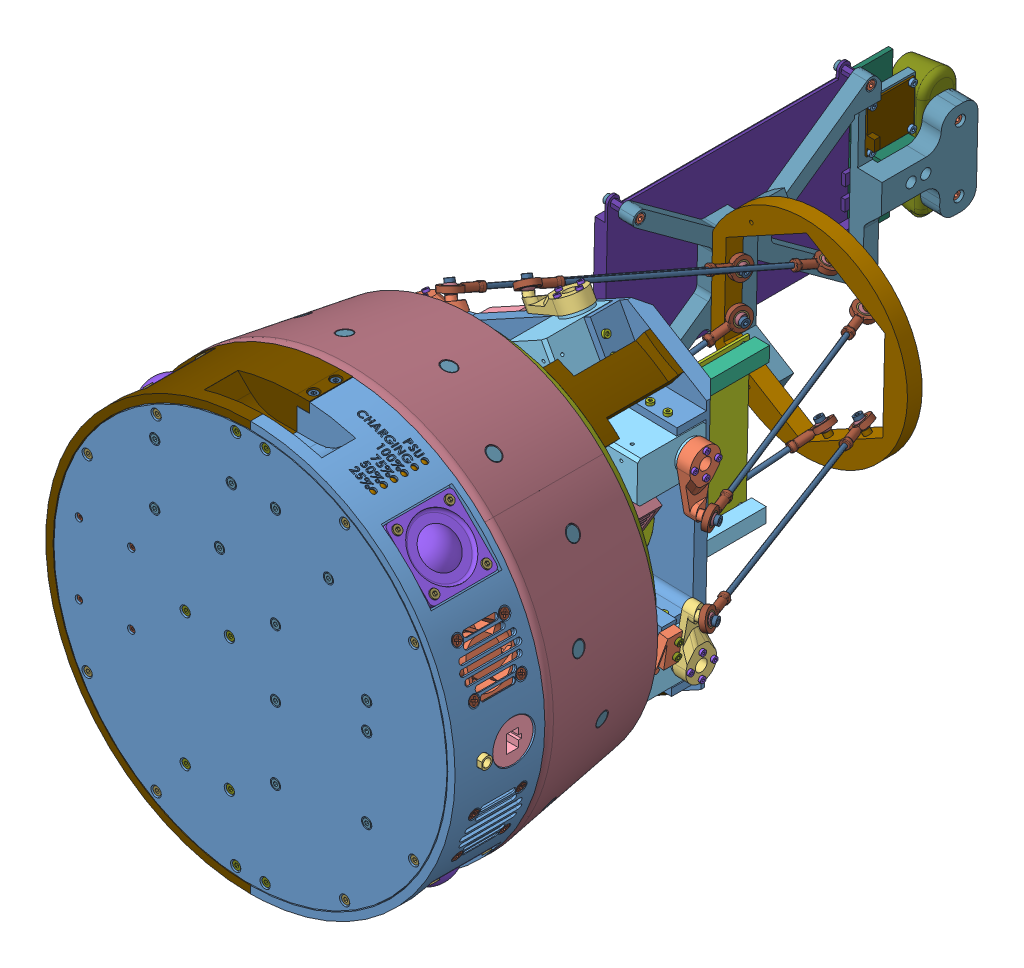
SolidWorks assembly robot, configuration Défaut. Lengths in mm.
Overall size (396.47 396.47 545.77).
549 component instances, 74 part files, 32 mates.
Components (placement in the parent):
- base-1: base [Défaut] at (1.1221 6.1042 181.6948) size (396.47 396.47 151)
  - base disk-1: base disk [Défaut] at (-2.864 19.6864 20.1) size (267 267 64.2)
    - base disk-1: base disk [Défaut] at (-39.9498 -9.3034 266.18) size (267 267 4)
    - Adafruit MAX9744-1: Adafruit MAX9744 [Défaut] at (-138.6977 -9.3034 256.18) x (0 1 0) z (0 0 -1) size (56.74 43.64 13.6)
    - Adafruit MAX9744-2: Adafruit MAX9744 [Défaut] at (-138.6977 -9.3034 239.58) x (0 1 0) z (0 0 -1) size (56.74 43.64 13.6)
    - Battery charger RRC-PMM240-1: Battery charger RRC-PMM240 [Défaut] at (-49.1471 67.1868 256.18) x (0 -1 0) z (0 0 -1) size (57 70 12)
    - battery holder-1: battery holder [Défaut] at (-89.2498 0.6966 266.18) x (0 -1 0) z (1 0 0) size (100 10 40)
    - Battery RRC2054-2-1: Battery RRC2054-2 [Défaut] at (-78.6791 -10.7125 233.18) x (0 1 0) z (0 0 1) size (151 78 23)
    - ground loop noise isolator-1: ground loop noise isolator [Défaut] at (-101.4098 -100.3034 233.18) x (0 -1 0) z (1 0 0) size (20 20 60)
    - ground loop noise isolator-2: ground loop noise isolator [Défaut] at (-41.4098 -80.3034 233.18) x (0 0 1) z (-1 0 0) size (20 20 60)
    - psu control-1: psu control [Défaut] at (-26.9498 90.6966 256.18) x (0 -1 0) z (0 0 -1) size (90 70 19.1)
    - buck boost-2: buck boost [Défaut] at (-26.9498 -9.3034 229.58) x (0 -1 0) z (0 0 -1) size (80 70 23.6)
    - 732-12936-ND-1: 732-12936-ND [Défaut] at (-156.4777 14.8266 254.58) x (-0.923728 -0.383049 0) z (0 0 -1) size (4.6 4.17 20)
    - 732-12936-ND-2: 732-12936-ND [Défaut] at (-156.4777 -33.4334 254.58) x (-0.923728 -0.383049 0) z (0 0 -1) size (4.6 4.17 20)
    - 732-12936-ND-3: 732-12936-ND [Défaut] at (-120.9177 -33.4334 254.58) x (-0.923728 -0.383049 0) z (0 0 -1) size (4.6 4.17 20)
    - 732-12936-ND-4: 732-12936-ND [Défaut] at (-120.9177 14.8266 254.58) x (-0.923728 -0.383049 0) z (0 0 -1) size (4.6 4.17 20)
    - 732-12918-ND-1: 732-12918-ND [Défaut] at (-156.4777 14.8266 266.18) x (-0.923728 -0.383049 0) z (0 0 -1) size (4.6 4.17 15)
    - 732-12918-ND-2: 732-12918-ND [Défaut] at (-120.9177 14.8266 266.18) x (-0.923728 -0.383049 0) z (0 0 -1) size (4.6 4.17 15)
    - 732-12918-ND-3: 732-12918-ND [Défaut] at (-120.9177 -33.4334 266.18) x (-0.923728 -0.383049 0) z (0 0 -1) size (4.6 4.17 15)
    - 732-12918-ND-4: 732-12918-ND [Défaut] at (-156.4777 -33.4334 266.18) x (-0.923728 -0.383049 0) z (0 0 -1) size (4.6 4.17 15)
    - M2x5mm socket-1: M2x5mm socket [Défaut] at (-156.4777 -33.4334 262.68) size (3.8 3.8 6.6)
    - M2x5mm socket-2: M2x5mm socket [Défaut] at (-120.9177 -33.4334 262.68) size (3.8 3.8 6.6)
    - M2x5mm socket-3: M2x5mm socket [Défaut] at (-156.4777 14.8266 262.68) size (3.8 3.8 6.6)
    - M2x5mm socket-4: M2x5mm socket [Défaut] at (-120.9177 14.8266 262.68) size (3.8 3.8 6.6)
    - M2 nut-1: M2 nut [Défaut] at (-156.4777 14.8266 237.98) x (-0.923728 -0.383049 0) z (0 0 -1) size (4.62 4 1.6)
    - M2 nut-2: M2 nut [Défaut] at (-156.4777 -33.4334 237.98) x (-0.923728 -0.383049 0) z (0 0 -1) size (4.62 4 1.6)
    - M2 nut-3: M2 nut [Défaut] at (-120.9177 -33.4334 237.98) x (-0.923728 -0.383049 0) z (0 0 -1) size (4.62 4 1.6)
    - M2 nut-4: M2 nut [Défaut] at (-120.9177 14.8266 237.98) x (-0.923728 -0.383049 0) z (0 0 -1) size (4.62 4 1.6)
    - 36-24337-ND-1: 36-24337-ND [Défaut] at (-104.9498 86.6966 266.18) x (-0.923728 -0.383049 0) z (0 0 -1) size (5.77 5 18)
    - 36-24337-ND-2: 36-24337-ND [Défaut] at (-104.9498 45.6966 266.18) x (-0.923728 -0.383049 0) z (0 0 -1) size (5.77 5 18)
    - 36-24337-ND-3: 36-24337-ND [Défaut] at (-60.9498 44.6966 266.18) x (-0.923728 -0.383049 0) z (0 0 -1) size (5.77 5 18)
    - 36-24337-ND-4: 36-24337-ND [Défaut] at (-52.9498 86.6966 266.18) x (-0.923728 -0.383049 0) z (0 0 -1) size (5.77 5 18)
    - M3x5mm socket-1: M3x5mm socket [Défaut] at (-104.9498 86.6966 262.18) size (5.5 5.5 8)
    - M3x5mm socket-2: M3x5mm socket [Défaut] at (-104.9498 45.6966 262.18) size (5.5 5.5 8)
    - M3x5mm socket-3: M3x5mm socket [Défaut] at (-60.9498 44.6966 262.18) size (5.5 5.5 8)
    - M3x5mm socket-4: M3x5mm socket [Défaut] at (-52.9498 86.6966 262.18) size (5.5 5.5 8)
    - M3 nut-1: M3 nut [Défaut] at (-104.9498 86.6966 254.18) x (-0.923728 -0.383049 0) z (0 0 -1) size (6.35 5.5 2.4)
    - M3 nut-2: M3 nut [Défaut] at (-104.9498 45.6966 254.18) x (-0.923728 -0.383049 0) z (0 0 -1) size (6.35 5.5 2.4)
    - M3 nut-3: M3 nut [Défaut] at (-60.9498 44.6966 254.18) x (-0.923728 -0.383049 0) z (0 0 -1) size (6.35 5.5 2.4)
    - M3 nut-4: M3 nut [Défaut] at (-52.9498 86.6966 254.18) x (-0.923728 -0.383049 0) z (0 0 -1) size (6.35 5.5 2.4)
    - M3x5mm plastic-1: M3x5mm plastic [Défaut] at (-84.2498 -94.3034 262.18) size (5.5 5.5 7.3)
    - M3x5mm plastic-2: M3x5mm plastic [Défaut] at (-84.2498 -4.3034 262.18) size (5.5 5.5 7.3)
    - M3x5mm plastic-3: M3x5mm plastic [Défaut] at (-54.2498 -94.3034 262.18) size (5.5 5.5 7.3)
    - M3x5mm plastic-4: M3x5mm plastic [Défaut] at (-54.2498 -4.3034 262.18) size (5.5 5.5 7.3)
    - 36-24337-ND-5: 36-24337-ND [Défaut] at (-22.9498 86.6966 266.18) x (-0.923728 -0.383049 0) z (0 0 -1) size (5.77 5 18)
    - 36-24337-ND-6: 36-24337-ND [Défaut] at (-22.9498 18.6966 266.18) x (-1 0 0) z (0 0 -1) size (5.77 5 18)
    - 36-24337-ND-7: 36-24337-ND [Défaut] at (13.0502 63.6966 266.18) x (-0.923728 -0.383049 0) z (0 0 -1) size (5.77 5 18)
    - 36-24337-ND-8: 36-24337-ND [Défaut] at (39.0502 4.6966 266.18) x (-1 0 0) z (0 0 -1) size (5.77 5 18)
    - M3x5mm socket-5: M3x5mm socket [Défaut] at (-22.9498 86.6966 262.18) size (5.5 5.5 8)
    - M3x5mm socket-6: M3x5mm socket [Défaut] at (13.0502 63.6966 262.18) size (5.5 5.5 8)
    - M3x5mm socket-7: M3x5mm socket [Défaut] at (39.0502 4.6966 262.18) size (5.5 5.5 8)
    - M3x5mm socket-8: M3x5mm socket [Défaut] at (-22.9498 18.6966 262.18) size (5.5 5.5 8)
    - M3 nut-5: M3 nut [Défaut] at (-22.9498 86.6966 252.18) size (6.35 5.5 2.4)
    - M3 nut-6: M3 nut [Défaut] at (13.0502 63.6966 252.18) size (6.35 5.5 2.4)
    - M3 nut-7: M3 nut [Défaut] at (-22.9498 18.6966 252.18) size (6.35 5.5 2.4)
    - M3 nut-8: M3 nut [Défaut] at (39.0502 4.6966 252.18) size (6.35 5.5 2.4)
    - 36-24337-ND-9: 36-24337-ND [Défaut] at (-22.9498 -26.3034 266.18) x (-0.923728 -0.383049 0) z (0 0 -1) size (5.77 5 18)
    - 36-24337-ND-10: 36-24337-ND [Défaut] at (-22.9498 -75.3034 266.18) x (-0.923728 -0.383049 0) z (0 0 -1) size (5.77 5 18)
    - 36-24337-ND-11: 36-24337-ND [Défaut] at (39.0502 -67.3034 266.18) x (-0.923728 -0.383049 0) z (0 0 -1) size (5.77 5 18)
    - 36-24337-ND-12: 36-24337-ND [Défaut] at (39.0502 -13.3034 266.18) x (-0.923728 -0.383049 0) z (0 0 -1) size (5.77 5 18)
    - M3x5mm socket-9: M3x5mm socket [Défaut] at (39.0502 -13.3034 262.18) x (0.878614 0.477533 0) z (0 0 1) size (5.5 5.5 8)
    - M3x5mm socket-10: M3x5mm socket [Défaut] at (39.0502 -67.3034 262.18) size (5.5 5.5 8)
    - M3x5mm socket-11: M3x5mm socket [Défaut] at (-22.9498 -75.3034 262.18) size (5.5 5.5 8)
    - M3x5mm socket-12: M3x5mm socket [Défaut] at (-22.9498 -26.3034 262.18) size (5.5 5.5 8)
    - buck boost-1: buck boost [Défaut] at (-26.9498 -9.3034 256.18) x (0 -1 0) z (0 0 -1) size (80 70 23.6)
    - 36-24342-ND-1: 36-24342-ND [Défaut] at (-22.9498 -26.3034 254.58) x (1 0 0) z (0 0 -1) size (5.77 5 33)
    - 36-24342-ND-2: 36-24342-ND [Défaut] at (-22.9498 -75.3034 254.58) x (1 0 0) z (0 0 -1) size (5.77 5 33)
    - 36-24342-ND-3: 36-24342-ND [Défaut] at (39.0502 -13.3034 254.58) x (1 0 0) z (0 0 -1) size (5.77 5 33)
    - 36-24342-ND-4: 36-24342-ND [Défaut] at (39.0502 -67.3034 254.58) x (1 0 0) z (0 0 -1) size (5.77 5 33)
    - M3 nut-9: M3 nut [Défaut] at (39.0502 -13.3034 225.58) size (6.35 5.5 2.4)
    - M3 nut-10: M3 nut [Défaut] at (-22.9498 -26.3034 225.58) size (6.35 5.5 2.4)
    - M3 nut-11: M3 nut [Défaut] at (-22.9498 -75.3034 225.58) size (6.35 5.5 2.4)
    - M3 nut-12: M3 nut [Défaut] at (39.0502 -67.3034 225.58) size (6.35 5.5 2.4)
  - base audio-1: base audio [Défaut] at (-124.8488 -53.3863 500.7234) x (-0.707186 -0.707027 0) z (0 0 -1) size (280.35 280.35 66)
    - base audio 1-1: base audio 1 [Défaut] at (-103.1006 -12.9042 210.4434) size (243.44 238.72 66)
    - base audio 2-1: base audio 2 [Défaut] at (-103.1006 -12.9042 210.4434) size (237.43 237.43 66)
    - Noctua NF-A4X20-1: Noctua NF-A4X20 [Défaut] at (-150.4017 -116.7762 243.4434) x (0.910081 -0.414431 0) z (-0.414431 -0.910081 0) size (39.9 39.9 19.95)
    - Noctua NF-A4X20-2: Noctua NF-A4X20 [Défaut] at (-206.9702 -60.2108 243.4434) x (0 0 1) z (-0.910059 -0.414479 0) size (39.9 39.9 19.95)
    - SC2073-ND-1: SC2073-ND [Défaut] at (-196.9231 -106.7266 228.7434) x (-0.707107 0.707107 0) z (-0.707107 -0.707107 0) size (11.94 11.94 36.36)
    - RJ45 connector-1: RJ45 connector [Défaut] at (-200.7415 -110.545 250.4434) x (-0.707107 0.707107 0) z (0.707107 0.707107 0) size (27.9 27.9 35.9)
    - switch-1: switch [Défaut] at (-57.531 -144.4179 258.9434) x (0.944885 0.327404 0) z (-0.327404 0.944885 0) size (20.75 14.7 24.67)
    - Micro USB B (Adafruit 4217)-1: Micro USB B (Adafruit 4217) [Défaut] at (-68.5317 -112.6698 234.4434) x (0.944885 0.327404 0) z (0 0 -1) size (28 33.5 28)
    - Micro USB B nut (Adafruit 4217)-1: Micro USB B nut (Adafruit 4217) [Défaut] at (-60.3466 -136.2919 234.4434) x (0.892807 0.309359 0.327404) z (-0.327404 0.944885 0) size (30.02 30.02 8)
    - Dayton Audio DMA45-8-1: Dayton Audio DMA45-8 [Défaut] at (-103.1023 -147.0792 243.4417) x (1 0 0) z (0 -1 0) size (46 46 32.1)
    - LED 5mm-1: LED 5mm [Défaut] at (-235.7284 26.7015 262.9434) x (-0.32152 -0.927903 0.188734) z (0.944885 -0.327404 0) size (5.5 5.5 18.7)
    - LED 5mm-2: LED 5mm [Défaut] at (-235.7284 26.7015 227.9434) x (-0.107193 -0.309359 0.944885) z (0.944885 -0.327404 0) size (5.5 5.5 18.7)
    - LED 5mm-3: LED 5mm [Défaut] at (-235.7284 26.7015 255.9434) x (-0.107193 -0.309359 0.944885) z (0.944885 -0.327404 0) size (5.5 5.5 18.7)
    - LED 5mm-4: LED 5mm [Défaut] at (-235.7284 26.7015 248.9434) x (-0.107193 -0.309359 0.944885) z (0.944885 -0.327404 0) size (5.5 5.5 18.7)
    - LED 5mm-5: LED 5mm [Défaut] at (-235.7284 26.7015 241.9434) x (-0.107193 -0.309359 0.944885) z (0.944885 -0.327404 0) size (5.5 5.5 18.7)
    - LED 5mm-6: LED 5mm [Défaut] at (-235.7284 26.7015 234.9434) x (-0.107193 -0.309359 0.944885) z (0.944885 -0.327404 0) size (5.5 5.5 18.7)
    - M3x12mm plastic-1: M3x12mm plastic [Défaut] at (-193.8472 71.832 264.1934) x (0.5 0.5 0.707107) z (-0.707107 0.707107 0) size (5.5 5.5 14.3)
    - M3x12mm plastic-2: M3x12mm plastic [Défaut] at (-193.8472 71.832 249.1934) x (0.5 0.5 0.707107) z (-0.707107 0.707107 0) size (5.5 5.5 14.3)
    - M3x12mm plastic-3: M3x12mm plastic [Défaut] at (-18.3645 -103.6507 264.1934) x (0.5 0.5 -0.707107) z (0.707107 -0.707107 0) size (5.5 5.5 14.3)
    - M3x12mm plastic-4: M3x12mm plastic [Défaut] at (-18.3645 -103.6507 249.1934) x (0.5 0.5 -0.707107) z (0.707107 -0.707107 0) size (5.5 5.5 14.3)
    - fan screw-1: fan screw [Défaut] at (-226.7522 -51.6391 259.4434) x (-0.171793 0.377201 -0.910059) z (-0.910059 -0.414479 0) size (6.3 6.3 9.5)
    - fan screw-2: fan screw [Défaut] at (-213.4889 -80.7609 259.4434) x (-0.171793 0.377201 -0.910059) z (-0.910059 -0.414479 0) size (6.3 6.3 9.5)
    - fan screw-3: fan screw [Défaut] at (-213.4889 -80.7609 227.4434) x (-0.171793 0.377201 -0.910059) z (-0.910059 -0.414479 0) size (6.3 6.3 9.5)
    - fan screw-4: fan screw [Défaut] at (-226.7522 -51.6391 227.4434) x (-0.171793 0.377201 -0.910059) z (-0.910059 -0.414479 0) size (6.3 6.3 9.5)
    - fan screw-5: fan screw [Défaut] at (-170.9515 -123.296 259.4434) x (-0.828247 0.377165 -0.414431) z (-0.414431 -0.910081 0) size (6.3 6.3 9.5)
    - fan screw-6: fan screw [Défaut] at (-141.8289 -136.5578 259.4434) x (-0.828247 0.377165 -0.414431) z (-0.414431 -0.910081 0) size (6.3 6.3 9.5)
    - fan screw-7: fan screw [Défaut] at (-141.8289 -136.5578 227.4434) x (-0.828247 0.377165 -0.414431) z (-0.414431 -0.910081 0) size (6.3 6.3 9.5)
    - fan screw-8: fan screw [Défaut] at (-170.9515 -123.296 227.4434) x (-0.828247 0.377165 -0.414431) z (-0.414431 -0.910081 0) size (6.3 6.3 9.5)
    - M3x8mm plastic-1: M3x8mm plastic [Défaut] at (-120.8506 -140.5792 261.1934) x (1 0 0) z (0 -1 0) size (5.5 5.5 10.3)
    - M3x8mm plastic-2: M3x8mm plastic [Défaut] at (-85.3506 -140.5792 261.1934) x (1 0 0) z (0 -1 0) size (5.5 5.5 10.3)
    - M3x8mm plastic-3: M3x8mm plastic [Défaut] at (-85.3506 -140.5792 225.6934) x (1 0 0) z (0 -1 0) size (5.5 5.5 10.3)
    - M3x8mm plastic-4: M3x8mm plastic [Défaut] at (-120.8506 -140.5792 225.6934) x (1 0 0) z (0 -1 0) size (5.5 5.5 10.3)
    - Dayton Audio DMA45-8-2: Dayton Audio DMA45-8 [Défaut] at (-237.2756 -12.9025 243.4417) x (0 -1 0) z (-1 0 0) size (46 46 32.1)
    - Dayton Audio DMA45-8-3: Dayton Audio DMA45-8 [Défaut] at (-103.099 121.2708 243.4417) x (-1 0 0) z (0 1 0) size (46 46 32.1)
    - Dayton Audio DMA45-8-4: Dayton Audio DMA45-8 [Défaut] at (31.0744 -12.9058 243.4417) x (0 1 0) z (1 0 0) size (46 46 32.1)
    - M3x8mm plastic-5: M3x8mm plastic [Défaut] at (-230.7756 -30.6542 261.1934) x (0 -1 0) z (-1 0 0) size (5.5 5.5 10.3)
    - M3x8mm plastic-6: M3x8mm plastic [Défaut] at (-120.8506 114.7708 261.1934) x (-1 0 0) z (0 1 0) size (5.5 5.5 10.3)
    - M3x8mm plastic-7: M3x8mm plastic [Défaut] at (24.5744 4.8458 261.1934) x (0 1 0) z (1 0 0) size (5.5 5.5 10.3)
    - M3x8mm plastic-8: M3x8mm plastic [Défaut] at (-230.7756 -30.6542 225.6934) x (0 -1 0) z (-1 0 0) size (5.5 5.5 10.3)
    - M3x8mm plastic-9: M3x8mm plastic [Défaut] at (-120.8506 114.7708 225.6934) x (-1 0 0) z (0 1 0) size (5.5 5.5 10.3)
    - M3x8mm plastic-10: M3x8mm plastic [Défaut] at (24.5744 4.8458 225.6934) x (0 1 0) z (1 0 0) size (5.5 5.5 10.3)
    - M3x8mm plastic-11: M3x8mm plastic [Défaut] at (-230.7756 4.8458 225.6934) x (0 -1 0) z (-1 0 0) size (5.5 5.5 10.3)
    - M3x8mm plastic-12: M3x8mm plastic [Défaut] at (-85.3506 114.7708 225.6934) x (-1 0 0) z (0 1 0) size (5.5 5.5 10.3)
    - M3x8mm plastic-13: M3x8mm plastic [Défaut] at (24.5744 -30.6542 225.6934) x (0 1 0) z (1 0 0) size (5.5 5.5 10.3)
    - M3x8mm plastic-14: M3x8mm plastic [Défaut] at (-230.7756 4.8458 261.1934) x (0 -1 0) z (-1 0 0) size (5.5 5.5 10.3)
    - M3x8mm plastic-15: M3x8mm plastic [Défaut] at (-85.3506 114.7708 261.1934) x (-1 0 0) z (0 1 0) size (5.5 5.5 10.3)
    - M3x8mm plastic-16: M3x8mm plastic [Défaut] at (24.5744 -30.6542 261.1934) x (0 1 0) z (1 0 0) size (5.5 5.5 10.3)
  - base mic-1: base mic [Défaut] at (-214.4966 156.9011 204.7877) x (-0.707186 -0.707027 0) z (0.707027 -0.707186 0) size (278.29 90 278.29)
    - base mic-1: base mic [Défaut] at (-17.8194 -24.4923 225) size (144.15 90 139.15)
    - 8SoundsUSB Mic-1: 8SoundsUSB Mic [Défaut] at (-144.6796 -4.9406 189.57) x (-0.19509 0 0.980785) z (-0.96871 0.156434 -0.192688) size (25.4 23.4 21.48)
    - 8SoundsUSB Mic-2: 8SoundsUSB Mic [Défaut] at (-118.9932 13.8255 145.3709) x (-0.55557 0 0.83147) z (-0.821233 0.156434 -0.54873) size (25.4 23.4 21.48)
    - 16SoundsUSB-1: 16SoundsUSB [Défaut] at (-17.8193 -7.4923 225) x (1 0 0) z (0 -1 0) size (165.86 165.78 26.13)
    - M3x5mm plastic-1: M3x5mm plastic [Défaut] at (-150.2647 13.5556 208.8509) x (0.213207 0.127057 -0.96871) z (0.96871 -0.156434 0.192688) size (5.5 5.5 7.3)
    - M3x5mm plastic-2: M3x5mm plastic [Défaut] at (-146.3629 13.5556 189.2352) x (0.213207 0.127057 -0.96871) z (0.96871 -0.156434 0.192688) size (5.5 5.5 7.3)
    - M3x5mm plastic-3: M3x5mm plastic [Défaut] at (-153.0264 -4.2228 208.3016) x (0.213207 0.127057 -0.96871) z (0.96871 -0.156434 0.192688) size (5.5 5.5 7.3)
    - M3x5mm plastic-4: M3x5mm plastic [Défaut] at (-149.1246 -4.2228 188.6859) x (0.213207 0.127057 -0.96871) z (0.96871 -0.156434 0.192688) size (5.5 5.5 7.3)
    - M3x5mm plastic-5: M3x5mm plastic [Défaut] at (-131.5316 32.3217 161.0468) x (0.564531 0.082951 -0.821233) z (0.821233 -0.156434 0.54873) size (5.5 5.5 7.3)
    - M3x5mm plastic-6: M3x5mm plastic [Défaut] at (-120.4201 32.3217 144.4174) x (0.564531 0.082951 -0.821233) z (0.821233 -0.156434 0.54873) size (5.5 5.5 7.3)
    - M3x5mm plastic-7: M3x5mm plastic [Défaut] at (-122.7614 14.5433 142.8531) x (0.564531 0.082951 -0.821233) z (0.821233 -0.156434 0.54873) size (5.5 5.5 7.3)
    - M3x5mm plastic-8: M3x5mm plastic [Défaut] at (-133.8728 14.5433 159.4825) x (0.564531 0.082951 -0.821233) z (0.821233 -0.156434 0.54873) size (5.5 5.5 7.3)
    - M3x8mm plastic-1: M3x8mm plastic [Défaut] at (-71.1944 -13.8489 171.625) x (1 0 0) z (0 1 0) size (5.5 5.5 10.3)
    - M3x8mm plastic-2: M3x8mm plastic [Défaut] at (-71.1944 -13.8489 278.375) x (-1 0 0) z (0 1 0) size (5.5 5.5 10.3)
    - M3x8mm plastic-3: M3x8mm plastic [Défaut] at (35.5556 -13.8489 171.625) x (1 0 0) z (0 1 0) size (5.5 5.5 10.3)
    - M3x8mm plastic-4: M3x8mm plastic [Défaut] at (35.5556 -13.8489 278.375) x (1 0 0) z (0 1 0) size (5.5 5.5 10.3)
    - base mic-2: base mic [Défaut] at (-17.8194 -24.4923 225) x (0 0 -1) z (1 0 0) size (144.15 90 139.15)
    - base mic-3: base mic [Défaut] at (-17.8194 -24.4923 225) x (-1 0 0) z (0 0 -1) size (144.15 90 139.15)
    - base mic-4: base mic [Défaut] at (-17.8194 -24.4923 225) x (0 0 1) z (-1 0 0) size (144.15 90 139.15)
    - 8SoundsUSB Mic-5: 8SoundsUSB Mic [Défaut] at (-132.5759 -4.9406 289.651) x (0.55557 0 0.83147) z (-0.821233 0.156434 0.54873) size (25.4 23.4 21.48)
    - 8SoundsUSB Mic-6: 8SoundsUSB Mic [Défaut] at (-53.2494 -4.9406 351.8603) x (0.980785 0 0.19509) z (-0.192688 0.156434 0.96871) size (25.4 23.4 21.48)
    - 8SoundsUSB Mic-7: 8SoundsUSB Mic [Défaut] at (46.8316 -4.9406 339.7566) x (0.83147 0 -0.55557) z (0.54873 0.156434 0.821233) size (25.4 23.4 21.48)
    - 8SoundsUSB Mic-8: 8SoundsUSB Mic [Défaut] at (109.0409 -4.9406 260.43) x (0.19509 0 -0.980785) z (0.96871 0.156434 0.192688) size (25.4 23.4 21.48)
    - 8SoundsUSB Mic-9: 8SoundsUSB Mic [Défaut] at (96.9372 -4.9406 160.349) x (-0.55557 0 -0.83147) z (0.821233 0.156434 -0.54873) size (25.4 23.4 21.48)
    - 8SoundsUSB Mic-10: 8SoundsUSB Mic [Défaut] at (17.6106 -4.9406 98.1397) x (-0.980785 0 -0.19509) z (0.192688 0.156434 -0.96871) size (25.4 23.4 21.48)
    - 8SoundsUSB Mic-11: 8SoundsUSB Mic [Défaut] at (-82.4703 -4.9406 110.2434) x (-0.83147 0 0.55557) z (-0.54873 0.156434 -0.821233) size (25.4 23.4 21.48)
    - 8SoundsUSB Mic-12: 8SoundsUSB Mic [Défaut] at (-145.6663 13.8255 240.2344) x (0.19509 0 0.980785) z (-0.96871 0.156434 0.192688) size (25.4 23.4 21.48)
    - 8SoundsUSB Mic-13: 8SoundsUSB Mic [Défaut] at (-97.4484 13.8255 326.1738) x (0.83147 0 0.55557) z (-0.54873 0.156434 0.821233) size (25.4 23.4 21.48)
    - 8SoundsUSB Mic-14: 8SoundsUSB Mic [Défaut] at (-2.5849 13.8255 352.8469) x (0.980785 0 -0.19509) z (0.192688 0.156434 0.96871) size (25.4 23.4 21.48)
    - 8SoundsUSB Mic-15: 8SoundsUSB Mic [Défaut] at (83.3545 13.8255 304.6291) x (0.55557 0 -0.83147) z (0.821233 0.156434 0.54873) size (25.4 23.4 21.48)
    - 8SoundsUSB Mic-16: 8SoundsUSB Mic [Défaut] at (110.0276 13.8255 209.7656) x (-0.19509 0 -0.980785) z (0.96871 0.156434 -0.192688) size (25.4 23.4 21.48)
    - 8SoundsUSB Mic-17: 8SoundsUSB Mic [Défaut] at (61.8097 13.8255 123.8262) x (-0.83147 0 -0.55557) z (0.54873 0.156434 -0.821233) size (25.4 23.4 21.48)
    - 8SoundsUSB Mic-18: 8SoundsUSB Mic [Défaut] at (-33.0538 13.8255 97.1531) x (-0.980785 0 0.19509) z (-0.192688 0.156434 -0.96871) size (25.4 23.4 21.48)
    - M3x5mm plastic-17: M3x5mm plastic [Défaut] at (-134.0029 13.5556 290.6045) x (-0.534222 0.127057 -0.835741) z (0.821233 -0.156434 -0.54873) size (5.5 5.5 7.3)
    - M3x5mm plastic-18: M3x5mm plastic [Défaut] at (-53.5842 13.5556 353.5435) x (-0.96871 0.127057 -0.213207) z (0.192688 -0.156434 -0.96871) size (5.5 5.5 7.3)
    - M3x5mm plastic-19: M3x5mm plastic [Défaut] at (47.7851 13.5556 341.1835) x (-0.835741 0.127057 0.534222) z (-0.54873 -0.156434 -0.821233) size (5.5 5.5 7.3)
    - M3x5mm plastic-20: M3x5mm plastic [Défaut] at (110.7242 13.5556 260.7648) x (-0.213207 0.127057 0.96871) z (-0.96871 -0.156434 -0.192688) size (5.5 5.5 7.3)
    - M3x5mm plastic-21: M3x5mm plastic [Défaut] at (98.3642 13.5556 159.3955) x (0.534222 0.127057 0.835741) z (-0.821233 -0.156434 0.54873) size (5.5 5.5 7.3)
    - M3x5mm plastic-22: M3x5mm plastic [Défaut] at (17.9454 13.5556 96.4565) x (0.96871 0.127057 0.213207) z (-0.192688 -0.156434 0.96871) size (5.5 5.5 7.3)
    - M3x5mm plastic-23: M3x5mm plastic [Défaut] at (-83.4238 13.5556 108.8165) x (0.835741 0.127057 -0.534222) z (0.54873 -0.156434 0.821233) size (5.5 5.5 7.3)
    - M3x5mm plastic-24: M3x5mm plastic [Défaut] at (-125.2328 -4.2228 308.7982) x (-0.534222 0.127057 -0.835741) z (0.821233 -0.156434 -0.54873) size (5.5 5.5 7.3)
    - M3x5mm plastic-25: M3x5mm plastic [Défaut] at (-34.5178 -4.2228 360.207) x (-0.96871 0.127057 -0.213207) z (0.192688 -0.156434 -0.96871) size (5.5 5.5 7.3)
    - M3x5mm plastic-26: M3x5mm plastic [Défaut] at (65.9789 -4.2228 332.4134) x (-0.835741 0.127057 0.534222) z (-0.54873 -0.156434 -0.821233) size (5.5 5.5 7.3)
    - M3x5mm plastic-27: M3x5mm plastic [Défaut] at (117.3877 -4.2228 241.6984) x (-0.213207 0.127057 0.96871) z (-0.96871 -0.156434 -0.192688) size (5.5 5.5 7.3)
    - M3x5mm plastic-28: M3x5mm plastic [Défaut] at (89.594 -4.2228 141.2018) x (0.534222 0.127057 0.835741) z (-0.821233 -0.156434 0.54873) size (5.5 5.5 7.3)
    - M3x5mm plastic-29: M3x5mm plastic [Défaut] at (-1.1209 -4.2228 89.793) x (0.96871 0.127057 0.213207) z (-0.192688 -0.156434 0.96871) size (5.5 5.5 7.3)
    - M3x5mm plastic-30: M3x5mm plastic [Défaut] at (-101.6176 -4.2228 117.5866) x (0.835741 0.127057 -0.534222) z (0.54873 -0.156434 0.821233) size (5.5 5.5 7.3)
    - M3x5mm plastic-31: M3x5mm plastic [Défaut] at (-136.3442 -4.2228 292.1688) x (-0.534222 0.127057 -0.835741) z (0.821233 -0.156434 -0.54873) size (5.5 5.5 7.3)
    - M3x5mm plastic-32: M3x5mm plastic [Défaut] at (-54.1335 -4.2228 356.3052) x (-0.96871 0.127057 -0.213207) z (0.192688 -0.156434 -0.96871) size (5.5 5.5 7.3)
    - M3x5mm plastic-33: M3x5mm plastic [Défaut] at (49.3495 -4.2228 343.5248) x (-0.835741 0.127057 0.534222) z (-0.54873 -0.156434 -0.821233) size (5.5 5.5 7.3)
    - M3x5mm plastic-34: M3x5mm plastic [Défaut] at (113.4859 -4.2228 261.3141) x (-0.213207 0.127057 0.96871) z (-0.96871 -0.156434 -0.192688) size (5.5 5.5 7.3)
    - M3x5mm plastic-35: M3x5mm plastic [Défaut] at (100.7054 -4.2228 157.8312) x (0.534222 0.127057 0.835741) z (-0.821233 -0.156434 0.54873) size (5.5 5.5 7.3)
    - M3x5mm plastic-36: M3x5mm plastic [Défaut] at (18.4948 -4.2228 93.6948) x (0.96871 0.127057 0.213207) z (-0.192688 -0.156434 0.96871) size (5.5 5.5 7.3)
    - M3x5mm plastic-37: M3x5mm plastic [Défaut] at (-84.9882 -4.2228 106.4752) x (0.835741 0.127057 -0.534222) z (0.54873 -0.156434 0.821233) size (5.5 5.5 7.3)
    - M3x5mm plastic-38: M3x5mm plastic [Défaut] at (-143.4477 32.3217 260.1849) x (-0.181515 0.082951 -0.979883) z (0.96871 -0.156434 -0.192688) size (5.5 5.5 7.3)
    - M3x5mm plastic-39: M3x5mm plastic [Défaut] at (-81.7725 32.3217 338.7122) x (-0.821233 0.082951 -0.564531) z (0.54873 -0.156434 -0.821233) size (5.5 5.5 7.3)
    - M3x5mm plastic-40: M3x5mm plastic [Défaut] at (17.3656 32.3217 350.6284) x (-0.979883 0.082951 0.181515) z (-0.192688 -0.156434 -0.96871) size (5.5 5.5 7.3)
    - M3x5mm plastic-41: M3x5mm plastic [Défaut] at (95.8928 32.3217 288.9532) x (-0.564531 0.082951 0.821233) z (-0.821233 -0.156434 -0.54873) size (5.5 5.5 7.3)
    - M3x5mm plastic-42: M3x5mm plastic [Défaut] at (107.809 32.3217 189.8151) x (0.181515 0.082951 0.979883) z (-0.96871 -0.156434 0.192688) size (5.5 5.5 7.3)
    - M3x5mm plastic-43: M3x5mm plastic [Défaut] at (46.1338 32.3217 111.2878) x (0.821233 0.082951 0.564531) z (-0.54873 -0.156434 0.821233) size (5.5 5.5 7.3)
    - M3x5mm plastic-44: M3x5mm plastic [Défaut] at (-53.0043 32.3217 99.3716) x (0.979883 0.082951 -0.181515) z (0.192688 -0.156434 0.96871) size (5.5 5.5 7.3)
    - M3x5mm plastic-45: M3x5mm plastic [Défaut] at (-147.3495 32.3217 240.5692) x (-0.181515 0.082951 -0.979883) z (0.96871 -0.156434 -0.192688) size (5.5 5.5 7.3)
    - M3x5mm plastic-46: M3x5mm plastic [Défaut] at (-98.4019 32.3217 327.6008) x (-0.821233 0.082951 -0.564531) z (0.54873 -0.156434 -0.821233) size (5.5 5.5 7.3)
    - M3x5mm plastic-47: M3x5mm plastic [Défaut] at (-2.2501 32.3217 354.5302) x (-0.979883 0.082951 0.181515) z (-0.192688 -0.156434 -0.96871) size (5.5 5.5 7.3)
    - M3x5mm plastic-48: M3x5mm plastic [Défaut] at (84.7814 32.3217 305.5826) x (-0.564531 0.082951 0.821233) z (-0.821233 -0.156434 -0.54873) size (5.5 5.5 7.3)
    - M3x5mm plastic-49: M3x5mm plastic [Défaut] at (111.7108 32.3217 209.4308) x (0.181515 0.082951 0.979883) z (-0.96871 -0.156434 0.192688) size (5.5 5.5 7.3)
    - M3x5mm plastic-50: M3x5mm plastic [Défaut] at (62.7632 32.3217 122.3992) x (0.821233 0.082951 0.564531) z (-0.54873 -0.156434 0.821233) size (5.5 5.5 7.3)
    - M3x5mm plastic-51: M3x5mm plastic [Défaut] at (-33.3886 32.3217 95.4698) x (0.979883 0.082951 -0.181515) z (0.192688 -0.156434 0.96871) size (5.5 5.5 7.3)
    - M3x5mm plastic-52: M3x5mm plastic [Défaut] at (-150.1113 14.5433 241.1186) x (-0.181515 0.082951 -0.979883) z (0.96871 -0.156434 -0.192688) size (5.5 5.5 7.3)
    - M3x5mm plastic-53: M3x5mm plastic [Défaut] at (-99.9663 14.5433 329.9421) x (-0.821233 0.082951 -0.564531) z (0.54873 -0.156434 -0.821233) size (5.5 5.5 7.3)
    - M3x5mm plastic-54: M3x5mm plastic [Défaut] at (-1.7008 14.5433 357.2919) x (-0.979883 0.082951 0.181515) z (-0.192688 -0.156434 -0.96871) size (5.5 5.5 7.3)
    - M3x5mm plastic-55: M3x5mm plastic [Défaut] at (87.1227 14.5433 307.1469) x (-0.564531 0.082951 0.821233) z (-0.821233 -0.156434 -0.54873) size (5.5 5.5 7.3)
    - M3x5mm plastic-56: M3x5mm plastic [Défaut] at (114.4725 14.5433 208.8814) x (0.181515 0.082951 0.979883) z (-0.96871 -0.156434 0.192688) size (5.5 5.5 7.3)
    - M3x5mm plastic-57: M3x5mm plastic [Défaut] at (64.3276 14.5433 120.0579) x (0.821233 0.082951 0.564531) z (-0.54873 -0.156434 0.821233) size (5.5 5.5 7.3)
    - M3x5mm plastic-58: M3x5mm plastic [Défaut] at (-33.9379 14.5433 92.7081) x (0.979883 0.082951 -0.181515) z (0.192688 -0.156434 0.96871) size (5.5 5.5 7.3)
    - M3x5mm plastic-59: M3x5mm plastic [Défaut] at (-146.2094 14.5433 260.7343) x (-0.181515 0.082951 -0.979883) z (0.96871 -0.156434 -0.192688) size (5.5 5.5 7.3)
    - M3x5mm plastic-60: M3x5mm plastic [Défaut] at (-83.3369 14.5433 341.0535) x (-0.821233 0.082951 -0.564531) z (0.54873 -0.156434 -0.821233) size (5.5 5.5 7.3)
    - M3x5mm plastic-61: M3x5mm plastic [Défaut] at (17.9149 14.5433 353.3901) x (-0.979883 0.082951 0.181515) z (-0.192688 -0.156434 -0.96871) size (5.5 5.5 7.3)
    - M3x5mm plastic-62: M3x5mm plastic [Défaut] at (98.2341 14.5433 290.5175) x (-0.564531 0.082951 0.821233) z (-0.821233 -0.156434 -0.54873) size (5.5 5.5 7.3)
    - M3x5mm plastic-63: M3x5mm plastic [Défaut] at (110.5707 14.5433 189.2657) x (0.181515 0.082951 0.979883) z (-0.96871 -0.156434 0.192688) size (5.5 5.5 7.3)
    - M3x5mm plastic-64: M3x5mm plastic [Défaut] at (47.6982 14.5433 108.9465) x (0.821233 0.082951 0.564531) z (-0.54873 -0.156434 0.821233) size (5.5 5.5 7.3)
    - M3x5mm plastic-65: M3x5mm plastic [Défaut] at (-53.5536 14.5433 96.6099) x (0.979883 0.082951 -0.181515) z (0.192688 -0.156434 0.96871) size (5.5 5.5 7.3)
    - M3x5mm plastic-66: M3x5mm plastic [Défaut] at (-122.8915 13.5556 307.2338) x (-0.534222 0.127057 -0.835741) z (0.821233 -0.156434 -0.54873) size (5.5 5.5 7.3)
    - M3x5mm plastic-67: M3x5mm plastic [Défaut] at (-33.9685 13.5556 357.4453) x (-0.96871 0.127057 -0.213207) z (0.192688 -0.156434 -0.96871) size (5.5 5.5 7.3)
    - M3x5mm plastic-68: M3x5mm plastic [Défaut] at (64.4145 13.5556 330.0721) x (-0.835741 0.127057 0.534222) z (-0.54873 -0.156434 -0.821233) size (5.5 5.5 7.3)
    - M3x5mm plastic-69: M3x5mm plastic [Défaut] at (114.626 13.5556 241.1491) x (-0.213207 0.127057 0.96871) z (-0.96871 -0.156434 -0.192688) size (5.5 5.5 7.3)
    - M3x5mm plastic-70: M3x5mm plastic [Défaut] at (87.2528 13.5556 142.7662) x (0.534222 0.127057 0.835741) z (-0.821233 -0.156434 0.54873) size (5.5 5.5 7.3)
    - M3x5mm plastic-71: M3x5mm plastic [Défaut] at (-1.6703 13.5556 92.5547) x (0.96871 0.127057 0.213207) z (-0.192688 -0.156434 0.96871) size (5.5 5.5 7.3)
    - M3x5mm plastic-72: M3x5mm plastic [Défaut] at (-100.0532 13.5556 119.9279) x (0.835741 0.127057 -0.534222) z (0.54873 -0.156434 0.821233) size (5.5 5.5 7.3)
  - M3x5mm plastic-1: M3x5mm plastic [Défaut] at (-52.7995 138.0832 282.28) size (5.5 5.5 7.3)
  - M3x5mm plastic-2: M3x5mm plastic [Défaut] at (-32.7995 138.0809 282.28) size (5.5 5.5 7.3)
  - M3x5mm plastic-3: M3x5mm plastic [Défaut] at (-52.8282 -117.3149 282.28) size (5.5 5.5 7.3)
  - M3x5mm plastic-4: M3x5mm plastic [Défaut] at (-32.8282 -117.3172 282.28) size (5.5 5.5 7.3)
  - M3x8mm plastic-1: M3x8mm plastic [Défaut] at (-106.8463 121.3194 279.28) size (5.5 5.5 10.3)
  - M3x8mm plastic-2: M3x8mm plastic [Défaut] at (-153.7358 74.4405 279.28) size (5.5 5.5 10.3)
  - M3x8mm plastic-3: M3x8mm plastic [Défaut] at (-153.7502 -53.6495 279.28) size (5.5 5.5 10.3)
  - M3x8mm plastic-4: M3x8mm plastic [Défaut] at (-106.8713 -100.539 279.28) size (5.5 5.5 10.3)
  - M3x8mm plastic-5: M3x8mm plastic [Défaut] at (21.2187 -100.5534 279.28) size (5.5 5.5 10.3)
  - M3x8mm plastic-6: M3x8mm plastic [Défaut] at (68.1082 -53.6745 279.28) size (5.5 5.5 10.3)
  - M3x8mm plastic-7: M3x8mm plastic [Défaut] at (68.1226 74.4155 279.28) size (5.5 5.5 10.3)
  - M3x8mm plastic-8: M3x8mm plastic [Défaut] at (21.2437 121.305 279.28) size (5.5 5.5 10.3)
  - M3x12mm plastic-1: M3x12mm plastic [Défaut] at (17.5379 -94.1764 231.28) x (-1 0 0) z (0 0 -1) size (5.5 5.5 14.3)
  - M3x12mm plastic-2: M3x12mm plastic [Défaut] at (61.732 -49.9922 231.28) x (-1 0 0) z (0 0 -1) size (5.5 5.5 14.3)
  - M3x12mm plastic-3: M3x12mm plastic [Défaut] at (61.7456 70.7347 231.28) x (-1 0 0) z (0 0 -1) size (5.5 5.5 14.3)
  - M3x12mm plastic-4: M3x12mm plastic [Défaut] at (17.5614 114.9288 231.28) x (-1 0 0) z (0 0 -1) size (5.5 5.5 14.3)
  - M3x12mm plastic-5: M3x12mm plastic [Défaut] at (-103.1655 114.9424 231.28) x (-1 0 0) z (0 0 -1) size (5.5 5.5 14.3)
  - M3x12mm plastic-6: M3x12mm plastic [Défaut] at (-147.3596 70.7582 231.28) x (-1 0 0) z (0 0 -1) size (5.5 5.5 14.3)
  - M3x12mm plastic-7: M3x12mm plastic [Défaut] at (-147.3732 -49.9687 231.28) x (-1 0 0) z (0 0 -1) size (5.5 5.5 14.3)
  - M3x12mm plastic-8: M3x12mm plastic [Défaut] at (-103.189 -94.1628 231.28) x (-1 0 0) z (0 0 -1) size (5.5 5.5 14.3)
- torso bottom-1: torso bottom [Défaut] at (25.4759 42.6645 86.9748) x (0.877353 0.479845 0) z (0 0 1) size (344.67 344.67 133.9) (flexible)
  - torso bottom (external)-1: torso bottom (external) [Défaut] at (-71.4907 9.2633 223) size (228 228 10)
  - torso bottom (internal)-1: torso bottom (internal) [Défaut] at (-71.4907 9.2633 223) x (0.5 -0.866025 0) z (0 0 1) size (152.18 175.73 60)
  - stewart support-1: stewart support [Défaut] at (-71.4907 9.2633 223) x (-0.976296 0.21644 0) z (0 0 -1) size (48.18 32.37 60)
  - limit switch support-1: limit switch support [Défaut] at (-71.4907 9.2633 223) x (-0.601815 -0.798636 0) z (0 0 -1) size (25 23.53 10)
  - limit switch-1: limit switch [Défaut] at (23.8828 -68.5535 217) x (0.601815 0.798636 0) z (-0.798636 0.601815 0) size (20 16.7 6)
  - slip ring (SNM220A-24)-1: slip ring (SNM220A-24) [Défaut] at (-71.4907 9.2633 280.5) x (0.866025 -0.5 0) z (0 0 -1) size (44 44 66.3)
  - gear servo support-1: gear servo support [Défaut] at (-152.6589 -14.9621 269.3) x (-0.5 0.866025 0) z (0 0 -1) size (72.26 87.14 59)
    - gear servo support-1: gear servo support [Défaut] at (-19.6043 81.2564 46.3) size (55 65.3 38)
    - XL430-W250-T-1: XL430-W250-T [Défaut] at (-13.6043 18.2064 84.3) x (0 -1 0) z (0 0 -1) size (28.5 46.5 36)
    - torso bottom gear-1: torso bottom gear [Défaut] at (-25.6043 18.2064 25.3) x (0 1 0) z (0 0 1) size (72.37 72.26 23)
    - M2.5x8mm plastic-1: M2.5x8mm plastic [Défaut] at (-21.6043 6.9564 73.3) x (1 0 0) z (0 -1 0) size (4.5 4.5 9.9)
    - M2.5x8mm plastic-2: M2.5x8mm plastic [Défaut] at (2.3957 6.9564 73.3) x (1 0 0) z (0 -1 0) size (4.5 4.5 9.9)
    - M2.5x8mm plastic-3: M2.5x8mm plastic [Défaut] at (-21.6043 6.9564 61.3) x (1 0 0) z (0 -1 0) size (4.5 4.5 9.9)
    - M2.5x8mm plastic-4: M2.5x8mm plastic [Défaut] at (2.3957 6.9564 61.3) x (1 0 0) z (0 -1 0) size (4.5 4.5 9.9)
    - M2.5x8mm plastic-5: M2.5x8mm plastic [Défaut] at (-34.1043 10.2064 61.3) x (0 0 1) z (-1 0 0) size (4.5 4.5 9.9)
    - M2.5x8mm plastic-6: M2.5x8mm plastic [Défaut] at (-34.1043 26.2064 61.3) x (0 0 1) z (-1 0 0) size (4.5 4.5 9.9)
    - M2x12mm socket-1: M2x12mm socket [Défaut] at (-25.6043 26.2064 51.3) x (-0.923728 -0.383049 0) z (0 0 -1) size (3.8 3.8 13.6)
    - M2x12mm socket-2: M2x12mm socket [Défaut] at (-33.6043 18.2064 51.3) x (1 0 0) z (0 0 -1) size (3.8 3.8 13.6)
    - M2x12mm socket-3: M2x12mm socket [Défaut] at (-17.6043 18.2064 51.3) x (-0.923728 -0.383049 0) z (0 0 -1) size (3.8 3.8 13.6)
    - M2x12mm socket-4: M2x12mm socket [Défaut] at (-25.6043 10.2064 51.3) x (1 0 0) z (0 0 -1) size (3.8 3.8 13.6)
  - stewart support-2: stewart support [Défaut] at (-71.4907 9.2633 223) x (0.67559 0.737277 0) z (0 0 -1) size (48.18 32.37 60)
  - stewart support-3: stewart support [Défaut] at (-71.4907 9.2633 223) x (0.300706 -0.953717 0) z (0 0 -1) size (48.18 32.37 60)
  - torso bottom holder-1: torso bottom holder [Défaut] at (-170.4452 56.3841 246.9839) x (-1 0 0) z (0 -1 0) size (28.75 23 26.74)
    - torso bottom holder-1: torso bottom holder [Défaut] at (-16.159 -8.0161 32.1209) size (28.75 22 26.74)
    - 605zz-1: 605zz [Défaut] at (4.9075 -2.0161 24.2498) x (0.173648 0 0.984808) z (-0.984808 0 0.173648) size (14 14 5)
    - M5 washer-1: M5 washer [Défaut] at (-0.0165 -2.0161 25.118) x (0.173648 0 0.984808) z (-0.984808 0 0.173648) size (10 10 1.1)
    - M5 washer-2: M5 washer [Défaut] at (5.9908 -2.0161 24.0588) x (0.173648 0 0.984808) z (-0.984808 0 0.173648) size (10 10 1.1)
    - M5x16mm socket-1: M5x16mm socket [Défaut] at (9.5361 -2.0161 23.4336) x (-0.984808 0 0.173648) z (-0.120191 -0.72175 -0.681639) size (21 8.5 8.5)
  - torso bottom holder-2: torso bottom holder [Défaut] at (18.7943 71.3999 246.9839) x (0.5 0.866025 0) z (-0.866025 0.5 0) size (28.75 23 26.74)
    - torso bottom holder-1: torso bottom holder [Défaut] at (-16.159 -8.0161 32.1209) size (28.75 22 26.74)
    - 605zz-1: 605zz [Défaut] at (4.9075 -2.0161 24.2498) x (0.173648 0 0.984808) z (-0.984808 0 0.173648) size (14 14 5)
    - M5 washer-1: M5 washer [Défaut] at (-0.0165 -2.0161 25.118) x (0.173648 0 0.984808) z (-0.984808 0 0.173648) size (10 10 1.1)
    - M5 washer-2: M5 washer [Défaut] at (5.9908 -2.0161 24.0588) x (0.173648 0 0.984808) z (-0.984808 0 0.173648) size (10 10 1.1)
    - M5x16mm socket-1: M5x16mm socket [Défaut] at (9.5361 -2.0161 23.4336) x (-0.984808 0 0.173648) z (-0.120191 -0.72175 -0.681639) size (21 8.5 8.5)
  - torso bottom holder-3: torso bottom holder [Défaut] at (-62.8214 -99.9942 246.9839) x (0.5 -0.866025 0) z (0.866025 0.5 0) size (28.75 23 26.74)
    - torso bottom holder-1: torso bottom holder [Défaut] at (-16.159 -8.0161 32.1209) size (28.75 22 26.74)
    - 605zz-1: 605zz [Défaut] at (4.9075 -2.0161 24.2498) x (0.173648 0 0.984808) z (-0.984808 0 0.173648) size (14 14 5)
    - M5 washer-1: M5 washer [Défaut] at (-0.0165 -2.0161 25.118) x (0.173648 0 0.984808) z (-0.984808 0 0.173648) size (10 10 1.1)
    - M5 washer-2: M5 washer [Défaut] at (5.9908 -2.0161 24.0588) x (0.173648 0 0.984808) z (-0.984808 0 0.173648) size (10 10 1.1)
    - M5x16mm socket-1: M5x16mm socket [Défaut] at (9.5361 -2.0161 23.4336) x (-0.984808 0 0.173648) z (-0.120191 -0.72175 -0.681639) size (21 8.5 8.5)
  - Jetson AGX Xavier-1: Jetson AGX Xavier [Défaut] at (-63.7145 17.7944 238.7) x (0.5 -0.866025 0) z (0 0 -1) size (105 105 65.46)
  - base gear-1: base gear [Défaut] at (-71.4907 9.2633 244) x (-0.779138 -0.626852 0) z (0 0 -1) size (245 245 13.91)
  - 605zz-1: 605zz [Défaut] at (30.0593 9.2633 229) x (0 0 -1) z (1 0 0) size (14 14 5)
  - 605zz-5: 605zz [Défaut] at (-122.2657 -78.6816 229) x (0 0 -1) z (-0.5 -0.866025 0) size (14 14 5)
  - 605zz-6: 605zz [Défaut] at (-122.2657 97.2082 229) x (0 0 -1) z (-0.5 0.866025 0) size (14 14 5)
  - M5 washer-1: M5 washer [Défaut] at (35.0593 9.2633 229) x (0 0 -1) z (1 0 0) size (10 10 1.1)
  - M5 washer-6: M5 washer [Défaut] at (-124.7657 -83.0117 229) x (0 0 -1) z (-0.5 -0.866025 0) size (10 10 1.1)
  - M5 washer-7: M5 washer [Défaut] at (-124.7657 101.5383 229) x (0 0 -1) z (-0.5 0.866025 0) size (10 10 1.1)
  - M5 washer-2: M5 washer [Défaut] at (28.9593 9.2633 229) x (0 0 -1) z (1 0 0) size (10 10 1.1)
  - M5 washer-8: M5 washer [Défaut] at (-121.7157 -77.729 229) x (0 0 -1) z (-0.5 -0.866025 0) size (10 10 1.1)
  - M5 washer-9: M5 washer [Défaut] at (-121.7157 96.2555 229) x (0 0 -1) z (-0.5 0.866025 0) size (10 10 1.1)
  - M5x16mm socket-1: M5x16mm socket [Défaut] at (38.5093 9.2633 229) x (-1 0 0) z (0 0 1) size (21 8.5 8.5)
  - M5x16mm socket-2: M5x16mm socket [Défaut] at (-126.4907 -85.9995 229) x (0.5 0.866025 0) z (0 0 1) size (21 8.5 8.5)
  - M5x16mm socket-3: M5x16mm socket [Défaut] at (-126.4907 104.5261 229) x (0.5 -0.866025 0) z (0 0 1) size (21 8.5 8.5)
  - 605zz-2: 605zz [Défaut] at (-20.7657 -78.595 229) x (0.75 0.433013 -0.5) z (0.5 -0.866025 0) size (14 14 5)
  - 605zz-3: 605zz [Défaut] at (-172.9407 9.2633 229) x (0 -0.866025 -0.5) z (-1 0 0) size (14 14 5)
  - 605zz-4: 605zz [Défaut] at (-20.7657 97.1216 229) x (-0.75 0.433013 -0.5) z (0.5 0.866025 0) size (14 14 5)
  - M5 washer-3: M5 washer [Défaut] at (-21.3157 -77.6424 229) x (0.75 0.433013 -0.5) z (0.5 -0.866025 0) size (10 10 1.1)
  - M5 washer-10: M5 washer [Défaut] at (-171.8407 9.2633 229) x (0 -0.866025 -0.5) z (-1 0 0) size (10 10 1.1)
  - M5 washer-11: M5 washer [Défaut] at (-21.3157 96.1689 229) x (-0.75 0.433013 -0.5) z (0.5 0.866025 0) size (10 10 1.1)
  - M5 washer-4: M5 washer [Défaut] at (-18.2657 -82.9251 229) x (0.75 0.433013 -0.5) z (0.5 -0.866025 0) size (10 10 1.1)
  - M5 washer-12: M5 washer [Défaut] at (-177.9407 9.2633 229) x (0 -0.866025 -0.5) z (-1 0 0) size (10 10 1.1)
  - M5 washer-13: M5 washer [Défaut] at (-18.2657 101.4517 229) x (-0.75 0.433013 -0.5) z (0.5 0.866025 0) size (10 10 1.1)
  - M5x30mm socket-1: M5x30mm socket [Défaut] at (-183.1862 9.2633 229) x (1 0 0) z (0 0.563112 0.826381) size (35 8.5 8.5)
  - M5x30mm socket-2: M5x30mm socket [Défaut] at (-15.643 105.9944 229) x (-0.5 -0.866025 0) z (0.487669 -0.281556 0.826381) size (35 8.5 8.5)
  - M5x30mm socket-3: M5x30mm socket [Défaut] at (-15.643 -87.4678 229) x (-0.5 0.866025 0) z (-0.487669 -0.281556 0.826381) size (35 8.5 8.5)
  - M5 washer-5: M5 washer [Défaut] at (-153.1862 9.2633 229) x (0 -0.866025 -0.5) z (-1 0 0) size (10 10 1.1)
  - M5 washer-14: M5 washer [Défaut] at (-30.643 80.0136 229) x (-0.75 0.433013 -0.5) z (0.5 0.866025 0) size (10 10 1.1)
  - M5 washer-15: M5 washer [Défaut] at (-30.643 -61.4871 229) x (0.75 0.433013 -0.5) z (0.5 -0.866025 0) size (10 10 1.1)
  - M3x12mm plastic-7: M3x12mm plastic [Défaut] at (-54.3258 -93.3104 229) x (-0.923728 -0.383049 0) z (0 0 -1) size (5.5 5.5 14.3)
  - M3x12mm plastic-9: M3x12mm plastic [Défaut] at (-168.9047 45.6849 229) x (0.130134 0.991496 0) z (0 0 -1) size (5.5 5.5 14.3)
  - M3x12mm plastic-10: M3x12mm plastic [Défaut] at (8.7582 75.4154 229) x (0.793594 -0.608447 0) z (0 0 -1) size (5.5 5.5 14.3)
  - M3x12mm plastic-8: M3x12mm plastic [Défaut] at (-88.6557 -93.3104 229) x (-1 0 0) z (0 0 -1) size (5.5 5.5 14.3)
  - M3x12mm plastic-11: M3x12mm plastic [Défaut] at (-151.7397 75.4154 229) x (0.5 0.866025 0) z (0 0 -1) size (5.5 5.5 14.3)
  - M3x12mm plastic-12: M3x12mm plastic [Défaut] at (25.9232 45.6849 229) x (0.5 -0.866025 0) z (0 0 -1) size (5.5 5.5 14.3)
  - M3x12mm plastic-13: M3x12mm plastic [Défaut] at (15.2334 -48.1382 229) x (-1 0 0) z (0 0 -1) size (5.5 5.5 14.3)
  - M3x12mm plastic-14: M3x12mm plastic [Défaut] at (7.5915 -58.2793 229) x (-1 0 0) z (0 0 -1) size (5.5 5.5 14.3)
  - M2.5x12mm plastic-1: M2.5x12mm plastic [Défaut] at (20.0164 -53.7447 217) x (0.362181 0.480631 -0.798636) z (0.798636 -0.601815 0) size (4.5 4.5 13.9)
  - M2.5x12mm plastic-2: M2.5x12mm plastic [Défaut] at (14.2992 -61.3317 217) x (0.362181 0.480631 -0.798636) z (0.798636 -0.601815 0) size (4.5 4.5 13.9)
  - M5x10mm plastic-1: M5x10mm plastic [Défaut] at (-71.4907 -8.2367 272.9) x (-0.5 -0.866025 0) z (0 0 1) size (8.5 8.5 13.5)
  - M5x10mm plastic-2: M5x10mm plastic [Défaut] at (-86.6462 18.0133 272.9) x (-0.5 -0.866025 0) z (0 0 1) size (8.5 8.5 13.5)
  - M5x10mm plastic-3: M5x10mm plastic [Défaut] at (-56.3353 18.0133 272.9) x (-0.5 -0.866025 0) z (0 0 1) size (8.5 8.5 13.5)
  - M3x12mm plastic-15: M3x12mm plastic [Défaut] at (-170.2862 17.7633 228) x (0 0 -1) z (1 0 0) size (5.5 5.5 14.3)
  - M3x12mm plastic-30: M3x12mm plastic [Défaut] at (-29.4542 -80.5461 228) x (0 0 -1) z (-0.5 0.866025 0) size (5.5 5.5 14.3)
  - M3x12mm plastic-29: M3x12mm plastic [Défaut] at (-14.7318 90.5727 228) x (0 0 -1) z (-0.5 -0.866025 0) size (5.5 5.5 14.3)
  - M3x12mm plastic-16: M3x12mm plastic [Défaut] at (-170.2862 0.7633 228) x (0 0 -1) z (1 0 0) size (5.5 5.5 14.3)
  - M3x12mm plastic-28: M3x12mm plastic [Défaut] at (-14.7318 -72.0461 228) x (0 0 -1) z (-0.5 0.866025 0) size (5.5 5.5 14.3)
  - M3x12mm plastic-27: M3x12mm plastic [Défaut] at (-29.4542 99.0727 228) x (0 0 -1) z (-0.5 -0.866025 0) size (5.5 5.5 14.3)
  - M3x12mm plastic-17: M3x12mm plastic [Défaut] at (-170.8875 -36.5765 229) x (-1 0 0) z (0 0 -1) size (5.5 5.5 14.3)
  - M3x12mm plastic-18: M3x12mm plastic [Défaut] at (-160.8875 -53.897 229) x (-0.923728 -0.383049 0) z (0 0 -1) size (5.5 5.5 14.3)
  - M3x12mm plastic-19: M3x12mm plastic [Défaut] at (-152.2273 -48.897 229) x (-0.923728 -0.383049 0) z (0 0 -1) size (5.5 5.5 14.3)
  - M3x12mm plastic-20: M3x12mm plastic [Défaut] at (-162.2273 -31.5765 229) x (-1 0 0) z (0 0 -1) size (5.5 5.5 14.3)
  - M3x12mm plastic-21: M3x12mm plastic [Défaut] at (-159.4762 20.2633 238) x (1 0 0) z (0 -1 0) size (5.5 5.5 14.3)
  - M3x12mm plastic-24: M3x12mm plastic [Défaut] at (-37.0243 -72.4344 238) x (-0.5 0.866025 0) z (0.866025 0.5 0) size (5.5 5.5 14.3)
  - M3x12mm plastic-23: M3x12mm plastic [Défaut] at (-17.9717 79.9609 238) x (-0.5 -0.866025 0) z (-0.866025 0.5 0) size (5.5 5.5 14.3)
  - M3x12mm plastic-22: M3x12mm plastic [Défaut] at (-159.4762 20.2633 245.78) x (1 0 0) z (0 -1 0) size (5.5 5.5 14.3)
  - M3x12mm plastic-26: M3x12mm plastic [Défaut] at (-37.0243 -72.4344 245.78) x (-0.5 0.866025 0) z (0.866025 0.5 0) size (5.5 5.5 14.3)
  - M3x12mm plastic-25: M3x12mm plastic [Défaut] at (-17.9717 79.9609 245.78) x (-0.5 -0.866025 0) z (-0.866025 0.5 0) size (5.5 5.5 14.3)
  - M3x55mm socket-1: M3x55mm socket [Défaut] at (-12.1356 -5.5428 204.7) size (5.5 5.5 58)
  - M3x55mm socket-2: M3x55mm socket [Défaut] at (-80.5516 -45.0428 204.7) size (5.5 5.5 58)
  - M3x55mm socket-3: M3x55mm socket [Défaut] at (-126.5516 34.6315 204.7) size (5.5 5.5 58)
  - M3x55mm socket-4: M3x55mm socket [Défaut] at (-58.1356 74.1315 204.7) size (5.5 5.5 58)
